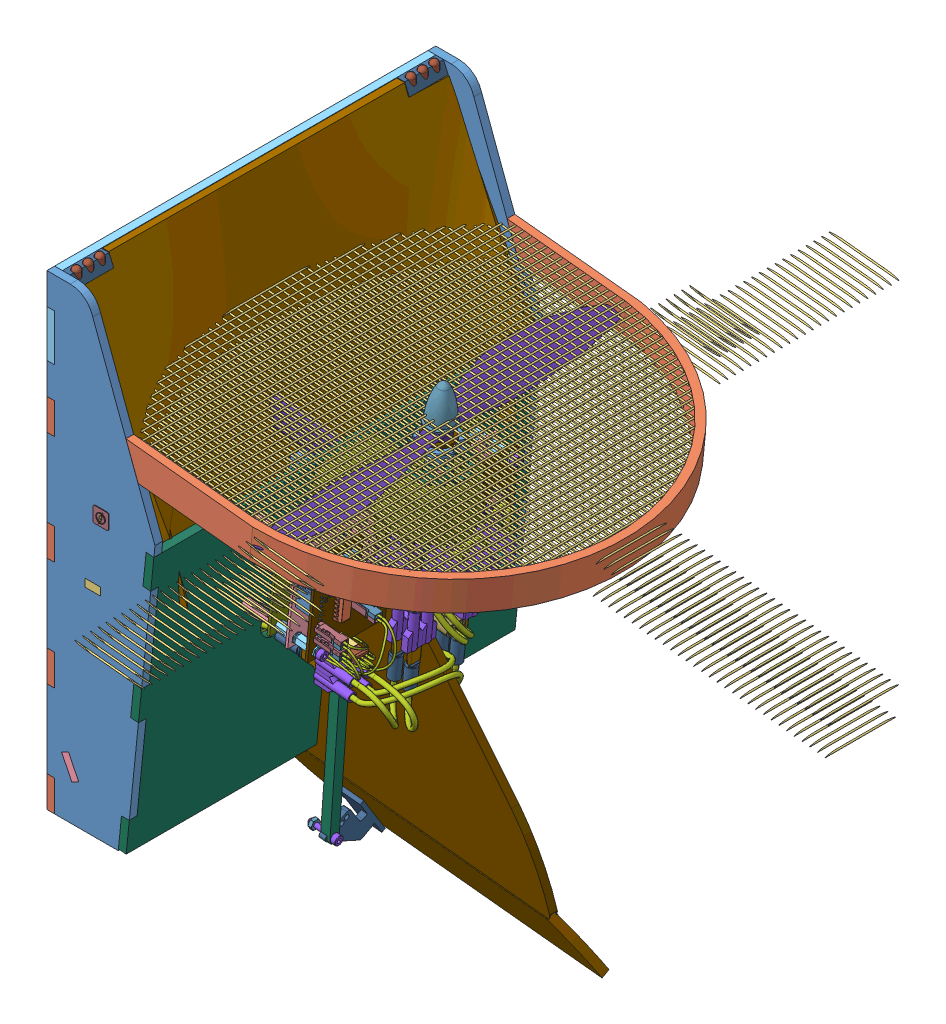
SolidWorks assembly AssTotaleSimu, configuration Défaut. Lengths in mm.
Overall size (323.53 384.35 253.57).
1760 component instances, 236 part files, 11 mates.
Components (placement in the parent):
- AssStructSimu-1: AssStructSimu [Défaut] at (-125.7658 -1.8483 624.6548) x (1 0 0) z (0 0 -1) size (323.53 326.04 251.6)
  - AssBase-1: AssBase [Défaut] at (36.5482 -71.0398 34.0612) size (266.84 303.75 251.6)
    - AssD-1: AssD [Défaut] at (39.0992 31.0201 8.5) size (69.5 300 22)
      - P1-1: P1 [Défaut] at (-95.5819 194.6656 377.5) size (69.5 300 5)
      - P5-1: P5 [Défaut] at (-100.5819 -35.3344 360.5) x (0 1 0) z (1 0 0) size (230 22 5)
    - AssG-1: AssG [Défaut] at (39.0992 31.0201 -236.5) size (69.5 300 22)
      - P1-1: P1 [Défaut] at (-95.5819 194.6656 377.5) size (69.5 300 5)
      - P5-1: P5 [Défaut] at (-95.5819 -35.3344 399.5) x (0 1 0) z (-1 0 0) size (230 22 5)
    - P7-1: P7 [Défaut] at (-1.4828 89.6857 370.5) x (0 0 -1) z (0 -1 0) size (250 54.5 5)
    - P4-1: P4 [Défaut] at (-63.2363 165.9323 386) x (0 0 -1) z (0.898794 -0.438371 0) size (250 60.5 66.27)
    - P3-1: P3 [Défaut] at (-56.4828 -74.3143 146) x (0 0 1) z (-1 0 0) size (250 70 5)
    - P4b-1: P4b [Défaut] at (-58.7423 163.7404 190) x (0 0 1) z (0.438371 0.898794 0) size (152 56 2)
    - battery-1: battery [Défaut] at (-39.0156 204.1861 197.5) x (0 0 1) z (0.898794 -0.438371 0) size (234.06 240.2 179.73)
    - socket head cap screw 4762_din-1: socket head cap screw 4762_din [EN ISO 4762 M3 x 10 - 10N] at (-27.7008 145.2627 193) x (0.438371 0.898794 0) z (0 0 -1) size (13 5.5 5.5)
    - socket head cap screw 4762_din-2: socket head cap screw 4762_din [EN ISO 4762 M3 x 10 - 10N] at (-27.7008 145.2627 339) x (0.438371 0.898794 0) z (-0.791285 0.385936 -0.474259) size (13 5.5 5.5)
    - socket head cap screw 4762_din-3: socket head cap screw 4762_din [EN ISO 4762 M3 x 10 - 10N] at (-42.0815 152.2766 339) x (0.438371 0.898794 0) z (-0.001489 0.000726 -0.999999) size (13 5.5 5.5)
    - socket head cap screw 4762_din-4: socket head cap screw 4762_din [EN ISO 4762 M3 x 10 - 10N] at (-42.0815 152.2766 193) x (0.438371 0.898794 0) z (-0.031331 0.015281 -0.999392) size (13 5.5 5.5)
    - P11-1: P11 [Défaut] at (-57.5734 -73.9703 146.7843) x (0.005072 0 0.999987) z (0.006197 0.999981 -0.000031) size (240 65 164)
    - AssPhare-1: AssPhare [Défaut] at (-52.8518 -67.6977 411) x (0 1 0) z (0 0 -1) size (43.2 8 27.06)
      - piece_led-1: piece_led [Défaut] at (-6.6166 -3.631 25) size (40.9 8 25)
      - LED 5mm-1: LED 5mm [Valor predeterminado] at (-0.1166 0.369 30) x (0 0 1) z (-1 0 0) size (5.5 6 35.8)
      - LED 5mm-2: LED 5mm [Valor predeterminado] at (-0.1166 0.369 37.5) x (0 0 1) z (-1 0 0) size (5.5 6 35.8)
      - LED 5mm-3: LED 5mm [Valor predeterminado] at (-0.1166 0.369 45) x (0 0 1) z (-1 0 0) size (5.5 6 35.8)
    - AssPhare-2: AssPhare [Défaut] at (-52.8518 -67.6977 196) x (0 1 0) z (0 0 -1) size (43.2 8 27.06)
      - piece_led-1: piece_led [Défaut] at (-6.6166 -3.631 25) size (40.9 8 25)
      - LED 5mm-1: LED 5mm [Valor predeterminado] at (-0.1166 0.369 30) x (0 0 1) z (-1 0 0) size (5.5 6 35.8)
      - LED 5mm-2: LED 5mm [Valor predeterminado] at (-0.1166 0.369 37.5) x (0 0 1) z (-1 0 0) size (5.5 6 35.8)
      - LED 5mm-3: LED 5mm [Valor predeterminado] at (-0.1166 0.369 45) x (0 0 1) z (-1 0 0) size (5.5 6 35.8)
    - AssLogo-1: AssLogo [Défaut] at (-27.8835 45.1673 148.1054) x (-1 0 0) z (0 0 -1) size (10 10 0.8)
      - logo1-1: logo1 [Défaut] at (-6.5271 -4.4734 6.5054) size (5.8 7.71 0.4)
      - logo2-1: logo2 [Défaut] at (-6.4007 -4.4815 7.1054) size (10 10 0.4)
    - AssLogo-2: AssLogo [Défaut] at (-25.082 45.1673 383.8946) size (10 10 0.8)
      - logo1-1: logo1 [Défaut] at (-6.5271 -4.4734 6.5054) size (5.8 7.71 0.4)
      - logo2-1: logo2 [Défaut] at (-6.4007 -4.4815 7.1054) size (10 10 0.4)
    - support2-1: support2 [Défaut] at (-61.5648 191.7124 276) x (-0.017452 -0.999848 0) z (0.999848 -0.017452 0) size (75 20 10) (hidden)
    - socket head cap screw 4762_din-5: socket head cap screw 4762_din [EN ISO 4762 M3 x 5 - 5N] at (-61.652 186.7132 269.3333) x (0.999848 -0.017452 0) z (-0.002158 -0.123615 0.992328) size (8 5.5 5.5)
    - socket head cap screw 4762_din-6: socket head cap screw 4762_din [EN ISO 4762 M3 x 5 - 5N] at (-61.652 186.7132 262.6667) x (0.999848 -0.017452 0) z (0 0 1) size (8 5.5 5.5)
    - socket head cap screw 4762_din-7: socket head cap screw 4762_din [EN ISO 4762 M3 x 25 - 18N] at (-55.2963 121.0922 253) x (0 0 1) z (-1 0 0) size (28 5.5 5.5)
    - hex nut style 1 gradeab_din-1: hex nut style 1 gradeab_din [Hexagon Nut ISO 4032 - M3 - W - N] at (-55.2963 121.0922 276) x (-0.923728 -0.383049 0) z (0 0 -1) size (5.5 6.35 2.4)
  - AssToitMot-1: AssToitMot [Défaut] at (-168.5238 43.6961 238.494) x (0 0 -1) z (0.9948 0.101852 0) size (250 207.5 205)
    - AssToit-1: AssToit [Défaut] at (-23.0702 -16.5789 -3.7148) size (250 207.5 205)
      - P8-1: P8 [Défaut] at (-38.4971 122.5921 203.5) size (250 175 5)
      - P12-1: P12 [Défaut] at (-60.4971 -63.4079 265.5) x (1 0 0) z (0 -1 0) size (47.03 76.64 55)
      - P13-1: P13 [Défaut] at (-35.9971 -52.8579 208.5) x (0 0 1) z (-1 0 0) size (64 15.55 5)
      - P10_2-1: P10_2 [Défaut] at (-35.9971 111.5921 171) x (0 0 1) z (-1 0 0) size (188.5 117.6 5)
    - Parallax-Servo_DUMMY-1: Parallax-Servo_DUMMY [Défaut] at (-61.6002 -51.5207 216.6662) x (1 0 0) z (0 1 0) size (20.07 42.79 55.64)
    - socket head cap screw 4762_din-1: socket head cap screw 4762_din [EN ISO 4762 M2.5 x 5 - 5N] at (-51.9272 -76.4868 259.2852) x (0 -1 0) z (-0.546944 0 0.837169) size (7.5 4.5 4.5)
    - socket head cap screw 4762_din-2: socket head cap screw 4762_din [EN ISO 4762 M2.5 x 5 - 5N] at (-61.5672 -76.4868 268.9252) x (0 -1 0) z (-0.546944 0 0.837169) size (7.5 4.5 4.5)
    - socket head cap screw 4762_din-3: socket head cap screw 4762_din [EN ISO 4762 M2.5 x 5 - 5N] at (-71.2072 -76.4868 259.2852) x (0 -1 0) z (-0.546944 0 0.837169) size (7.5 4.5 4.5)
    - socket head cap screw 4762_din-4: socket head cap screw 4762_din [EN ISO 4762 M2.5 x 5 - 5N] at (-61.5672 -76.4868 249.6452) x (0 -1 0) z (-0.546944 0 0.837169) size (7.5 4.5 4.5)
    - AssPhare-1: AssPhare [Défaut] at (8.4328 83.3966 196.1542) x (0 -1 0) z (1 0 0) size (43.2 8 27.06)
      - piece_led-1: piece_led [Défaut] at (-6.6166 -3.631 25) size (40.9 8 25)
      - LED 5mm-1: LED 5mm [Valor predeterminado] at (-0.1166 0.369 30) x (0 0 1) z (-1 0 0) size (5.5 6 35.8)
      - LED 5mm-2: LED 5mm [Valor predeterminado] at (-0.1166 0.369 37.5) x (0 0 1) z (-1 0 0) size (5.5 6 35.8)
      - LED 5mm-3: LED 5mm [Valor predeterminado] at (-0.1166 0.369 45) x (0 0 1) z (-1 0 0) size (5.5 6 35.8)
    - AssPhare-2: AssPhare [Défaut] at (-206.5672 83.3966 196.1542) x (0 -1 0) z (1 0 0) size (43.2 8 27.06)
      - piece_led-1: piece_led [Défaut] at (-6.6166 -3.631 25) size (40.9 8 25)
      - LED 5mm-1: LED 5mm [Valor predeterminado] at (-0.1166 0.369 30) x (0 0 1) z (-1 0 0) size (5.5 6 35.8)
      - LED 5mm-2: LED 5mm [Valor predeterminado] at (-0.1166 0.369 37.5) x (0 0 1) z (-1 0 0) size (5.5 6 35.8)
      - LED 5mm-3: LED 5mm [Valor predeterminado] at (-0.1166 0.369 45) x (0 0 1) z (-1 0 0) size (5.5 6 35.8)
    - socket head cap screw 4762_din-5: socket head cap screw 4762_din [EN ISO 4762 M3 x 10 - 10N] at (-67.0672 -22.9368 210.2852) x (0 0 -1) z (1 0 0) size (13 5.5 5.5)
    - socket head cap screw 4762_din-6: socket head cap screw 4762_din [EN ISO 4762 M3 x 10 - 10N] at (-56.0672 -72.9868 210.2852) x (0 0 -1) z (1 0 0) size (13 5.5 5.5)
    - socket head cap screw 4762_din-7: socket head cap screw 4762_din [EN ISO 4762 M3 x 10 - 10N] at (-67.0672 -72.9868 210.2852) x (0 0 -1) z (1 0 0) size (13 5.5 5.5)
    - socket head cap screw 4762_din-8: socket head cap screw 4762_din [EN ISO 4762 M3 x 10 - 10N] at (-56.0672 -22.9368 210.2852) x (0 0 -1) z (1 0 0) size (13 5.5 5.5)
    - hex nut style 1 gradeab_din-1: hex nut style 1 gradeab_din [Hexagon Nut ISO 4032 - M3 - W - N] at (-67.0672 -72.9868 197.3852) x (-0.923728 -0.383049 0) z (0 0 -1) size (5.5 6.35 2.4)
    - hex nut style 1 gradeab_din-2: hex nut style 1 gradeab_din [Hexagon Nut ISO 4032 - M3 - W - N] at (-56.0672 -72.9868 199.7852) size (5.5 6.35 2.4)
    - hex nut style 1 gradeab_din-3: hex nut style 1 gradeab_din [Hexagon Nut ISO 4032 - M3 - W - N] at (-67.0672 -22.9368 199.7852) size (5.5 6.35 2.4)
    - hex nut style 1 gradeab_din-4: hex nut style 1 gradeab_din [Hexagon Nut ISO 4032 - M3 - W - N] at (-56.0672 -22.9368 199.7852) size (5.5 6.35 2.4)
  - AssProtec-1: AssProtec [Défaut] at (86.6746 190.4649 284.6351) x (0 0 -1) z (0.101852 -0.9948 0) size (250 237.46 20)
    - protec3c-1: protec3c [Défaut] at (-140.4261 -87.7568 240) size (250 197 20)
    - AssGrillage-1: AssGrillage [Défaut] at (-370.4609 -132.5428 258.3161) x (0 0 -1) z (1 0 0) size (2.02 237.05 250)
      - barreau-1: barreau [Défaut] at (-1.1839 0.254 200) size (1 1 400)
      - barreau-3: barreau [Défaut] at (-1.1839 5.254 200) size (1 1 400)
      - barreau-4: barreau [Défaut] at (-1.1839 10.254 200) size (1 1 400)
      - barreau-5: barreau [Défaut] at (-1.1839 15.254 200) size (1 1 400)
      - barreau-6: barreau [Défaut] at (-1.1839 20.254 200) size (1 1 400)
      - barreau-7: barreau [Défaut] at (-1.1839 25.254 200) size (1 1 400)
      - barreau-8: barreau [Défaut] at (-1.1839 30.254 200) size (1 1 400)
      - barreau-9: barreau [Défaut] at (-1.1839 35.254 200) size (1 1 400)
      - barreau-10: barreau [Défaut] at (-1.1839 40.254 200) size (1 1 400)
      - barreau-11: barreau [Défaut] at (-1.1839 45.254 200) size (1 1 400)
      - barreau-12: barreau [Défaut] at (-1.1839 50.254 200) size (1 1 400)
      - barreau-13: barreau [Défaut] at (-1.1839 55.254 200) size (1 1 400)
      - barreau-14: barreau [Défaut] at (-1.1839 60.254 200) size (1 1 400)
      - barreau-15: barreau [Défaut] at (-1.1839 65.254 200) size (1 1 400)
      - barreau-16: barreau [Défaut] at (-1.1839 70.254 200) size (1 1 400)
      - barreau-17: barreau [Défaut] at (-1.1839 75.254 200) size (1 1 400)
      - barreau-18: barreau [Défaut] at (-1.1839 80.254 200) size (1 1 400)
      - barreau-19: barreau [Défaut] at (-1.1839 85.254 200) size (1 1 400)
      - barreau-20: barreau [Défaut] at (-1.1839 90.254 200) size (1 1 400)
      - barreau-21: barreau [Défaut] at (-1.1839 95.254 200) size (1 1 400)
      - barreau-22: barreau [Défaut] at (-1.1839 100.254 200) size (1 1 400)
      - barreau-23: barreau [Défaut] at (-1.1839 105.254 200) size (1 1 400)
      - barreau-24: barreau [Défaut] at (-1.1839 110.254 200) size (1 1 400)
      - barreau-25: barreau [Défaut] at (-1.1839 115.254 200) size (1 1 400)
      - barreau-26: barreau [Défaut] at (-1.1839 120.254 200) size (1 1 400)
      - barreau-27: barreau [Défaut] at (-1.1839 125.254 200) size (1 1 400)
      - barreau-28: barreau [Défaut] at (-1.1839 130.254 200) size (1 1 400)
      - barreau-29: barreau [Défaut] at (-1.1839 135.254 200) size (1 1 400)
      - barreau-30: barreau [Défaut] at (-1.1839 140.254 200) size (1 1 400)
      - barreau-31: barreau [Défaut] at (-1.1839 145.254 200) size (1 1 400)
      - barreau-32: barreau [Défaut] at (-1.1839 150.254 200) size (1 1 400)
      - barreau-33: barreau [Défaut] at (-1.1839 155.254 200) size (1 1 400)
      - barreau-34: barreau [Défaut] at (-1.1839 160.254 200) size (1 1 400)
      - barreau-35: barreau [Défaut] at (-1.1839 165.254 200) size (1 1 400)
      - barreau-36: barreau [Défaut] at (-1.1839 170.254 200) size (1 1 400)
      - barreau-37: barreau [Défaut] at (-1.1839 175.254 200) size (1 1 400)
      - barreau-38: barreau [Défaut] at (-1.1839 180.254 200) size (1 1 400)
      - barreau-39: barreau [Défaut] at (-1.1839 185.254 200) size (1 1 400)
      - barreau-40: barreau [Défaut] at (-1.1839 190.254 200) size (1 1 400)
      - barreau-41: barreau [Défaut] at (-1.1839 195.254 200) size (1 1 400)
      - barreau-42: barreau [Défaut] at (-0.1839 -1.5314 598.7823) x (0.998922 0 0.04641) z (0 1 0) size (1 1 400)
      - barreau-43: barreau [Défaut] at (-1.1839 200.254 200) size (1 1 400)
      - barreau-44: barreau [Défaut] at (-1.1839 205.254 200) size (1 1 400)
      - barreau-45: barreau [Défaut] at (-1.1839 210.254 200) size (1 1 400)
      - barreau-46: barreau [Défaut] at (-1.1839 215.254 200) size (1 1 400)
      - barreau-47: barreau [Défaut] at (-1.1839 220.254 200) size (1 1 400)
      - barreau-48: barreau [Défaut] at (-1.1839 225.254 200) size (1 1 400)
      - barreau-49: barreau [Défaut] at (-1.1839 230.254 200) size (1 1 400)
      - barreau-50: barreau [Défaut] at (-1.1839 235.254 200) size (1 1 400)
      - barreau-51: barreau [Défaut] at (-1.1839 240.254 200) size (1 1 400)
      - barreau-52: barreau [Défaut] at (-1.1839 245.254 200) size (1 1 400)
      - barreau-53: barreau [Défaut] at (-1.1839 250.254 200) size (1 1 400)
      - barreau-54: barreau [Défaut] at (-1.1839 255.254 200) size (1 1 400)
      - barreau-55: barreau [Défaut] at (-1.1839 260.254 200) size (1 1 400)
      - barreau-56: barreau [Défaut] at (-1.1839 265.254 200) size (1 1 400)
      - barreau-57: barreau [Défaut] at (-1.1839 270.254 200) size (1 1 400)
      - barreau-58: barreau [Défaut] at (-1.1839 275.254 200) size (1 1 400)
      - barreau-59: barreau [Défaut] at (-1.1839 280.254 200) size (1 1 400)
      - barreau-60: barreau [Défaut] at (-1.1839 285.254 200) size (1 1 400)
      - barreau-61: barreau [Défaut] at (-1.1839 290.254 200) size (1 1 400)
      - barreau-62: barreau [Défaut] at (-1.1839 295.254 200) size (1 1 400)
      - barreau-63: barreau [Défaut] at (-1.1839 300.254 200) size (1 1 400)
      - barreau-64: barreau [Défaut] at (-1.1839 305.254 200) size (1 1 400)
      - barreau-65: barreau [Défaut] at (-1.1839 310.254 200) size (1 1 400)
      - barreau-66: barreau [Défaut] at (-1.1839 315.254 200) size (1 1 400)
      - barreau-67: barreau [Défaut] at (-1.1839 320.254 200) size (1 1 400)
      - barreau-68: barreau [Défaut] at (-1.1839 325.254 200) size (1 1 400)
      - barreau-69: barreau [Défaut] at (-1.1839 330.254 200) size (1 1 400)
      - barreau-70: barreau [Défaut] at (-1.1839 335.254 200) size (1 1 400)
      - barreau-71: barreau [Défaut] at (-1.1839 340.254 200) size (1 1 400)
      - barreau-72: barreau [Défaut] at (-1.1839 345.254 200) size (1 1 400)
      - barreau-73: barreau [Défaut] at (-1.1839 350.254 200) size (1 1 400)
      - barreau-74: barreau [Défaut] at (-1.1839 355.254 200) size (1 1 400)
      - barreau-75: barreau [Défaut] at (-1.1839 360.254 200) size (1 1 400)
      - barreau-76: barreau [Défaut] at (-1.1839 365.254 200) size (1 1 400)
      - barreau-77: barreau [Défaut] at (-1.1839 370.254 200) size (1 1 400)
      - barreau-78: barreau [Défaut] at (-1.1839 375.254 200) size (1 1 400)
      - barreau-79: barreau [Défaut] at (-1.1839 380.254 200) size (1 1 400)
      - barreau-80: barreau [Défaut] at (-1.1839 385.254 200) size (1 1 400)
      - barreau-81: barreau [Défaut] at (-1.1839 390.254 200) size (1 1 400)
      - barreau-82: barreau [Défaut] at (-1.1839 395.254 200) size (1 1 400)
      - barreau-136: barreau [Défaut] at (-0.1839 -1.5314 593.7823) x (0.998922 0 0.04641) z (0 1 0) size (1 1 400)
      - barreau-137: barreau [Défaut] at (-0.1839 -1.5314 588.7823) x (0.998922 0 0.04641) z (0 1 0) size (1 1 400)
      - barreau-138: barreau [Défaut] at (-0.1839 -1.5314 583.7823) x (0.998922 0 0.04641) z (0 1 0) size (1 1 400)
      - barreau-139: barreau [Défaut] at (-0.1839 -1.5314 578.7823) x (0.998922 0 0.04641) z (0 1 0) size (1 1 400)
      - barreau-140: barreau [Défaut] at (-0.1839 -1.5314 573.7823) x (0.998922 0 0.04641) z (0 1 0) size (1 1 400)
      - barreau-141: barreau [Défaut] at (-0.1839 -1.5314 568.7823) x (0.998922 0 0.04641) z (0 1 0) size (1 1 400)
      - barreau-142: barreau [Défaut] at (-0.1839 -1.5314 563.7823) x (0.998922 0 0.04641) z (0 1 0) size (1 1 400)
      - barreau-143: barreau [Défaut] at (-0.1839 -1.5314 558.7823) x (0.998922 0 0.04641) z (0 1 0) size (1 1 400)
      - barreau-144: barreau [Défaut] at (-0.1839 -1.5314 553.7823) x (0.998922 0 0.04641) z (0 1 0) size (1 1 400)
      - barreau-145: barreau [Défaut] at (-0.1839 -1.5314 548.7823) x (0.998922 0 0.04641) z (0 1 0) size (1 1 400)
      - barreau-146: barreau [Défaut] at (-0.1839 -1.5314 543.7823) x (0.998922 0 0.04641) z (0 1 0) size (1 1 400)
      - barreau-147: barreau [Défaut] at (-0.1839 -1.5314 538.7823) x (0.998922 0 0.04641) z (0 1 0) size (1 1 400)
      - barreau-148: barreau [Défaut] at (-0.1839 -1.5314 533.7823) x (0.998922 0 0.04641) z (0 1 0) size (1 1 400)
      - barreau-149: barreau [Défaut] at (-0.1839 -1.5314 528.7823) x (0.998922 0 0.04641) z (0 1 0) size (1 1 400)
      - barreau-150: barreau [Défaut] at (-0.1839 -1.5314 523.7823) x (0.998922 0 0.04641) z (0 1 0) size (1 1 400)
      - barreau-151: barreau [Défaut] at (-0.1839 -1.5314 518.7823) x (0.998922 0 0.04641) z (0 1 0) size (1 1 400)
      - barreau-152: barreau [Défaut] at (-0.1839 -1.5314 513.7823) x (0.998922 0 0.04641) z (0 1 0) size (1 1 400)
      - barreau-153: barreau [Défaut] at (-0.1839 -1.5314 508.7823) x (0.998922 0 0.04641) z (0 1 0) size (1 1 400)
      - barreau-154: barreau [Défaut] at (-0.1839 -1.5314 503.7823) x (0.998922 0 0.04641) z (0 1 0) size (1 1 400)
      - barreau-155: barreau [Défaut] at (-0.1839 -1.5314 498.7823) x (0.998922 0 0.04641) z (0 1 0) size (1 1 400)
      - barreau-156: barreau [Défaut] at (-0.1839 -1.5314 493.7823) x (0.998922 0 0.04641) z (0 1 0) size (1 1 400)
      - barreau-157: barreau [Défaut] at (-0.1839 -1.5314 488.7823) x (0.998922 0 0.04641) z (0 1 0) size (1 1 400)
      - barreau-158: barreau [Défaut] at (-0.1839 -1.5314 483.7823) x (0.998922 0 0.04641) z (0 1 0) size (1 1 400)
      - barreau-159: barreau [Défaut] at (-0.1839 -1.5314 478.7823) x (0.998922 0 0.04641) z (0 1 0) size (1 1 400)
      - barreau-160: barreau [Défaut] at (-0.1839 -1.5314 473.7823) x (0.998922 0 0.04641) z (0 1 0) size (1 1 400)
      - barreau-161: barreau [Défaut] at (-0.1839 -1.5314 468.7823) x (0.998922 0 0.04641) z (0 1 0) size (1 1 400)
      - barreau-162: barreau [Défaut] at (-0.1839 -1.5314 463.7823) x (0.998922 0 0.04641) z (0 1 0) size (1 1 400)
      - barreau-163: barreau [Défaut] at (-0.1839 -1.5314 458.7823) x (0.998922 0 0.04641) z (0 1 0) size (1 1 400)
      - barreau-164: barreau [Défaut] at (-0.1839 -1.5314 453.7823) x (0.998922 0 0.04641) z (0 1 0) size (1 1 400)
      - barreau-165: barreau [Défaut] at (-0.1839 -1.5314 448.7823) x (0.998922 0 0.04641) z (0 1 0) size (1 1 400)
      - barreau-166: barreau [Défaut] at (-0.1839 -1.5314 443.7823) x (0.998922 0 0.04641) z (0 1 0) size (1 1 400)
      - barreau-167: barreau [Défaut] at (-0.1839 -1.5314 438.7823) x (0.998922 0 0.04641) z (0 1 0) size (1 1 400)
      - barreau-168: barreau [Défaut] at (-0.1839 -1.5314 433.7823) x (0.998922 0 0.04641) z (0 1 0) size (1 1 400)
      - barreau-169: barreau [Défaut] at (-0.1839 -1.5314 428.7823) x (0.998922 0 0.04641) z (0 1 0) size (1 1 400)
      - barreau-170: barreau [Défaut] at (-0.1839 -1.5314 423.7823) x (0.998922 0 0.04641) z (0 1 0) size (1 1 400)
      - barreau-171: barreau [Défaut] at (-0.1839 -1.5314 418.7823) x (0.998922 0 0.04641) z (0 1 0) size (1 1 400)
      - barreau-172: barreau [Défaut] at (-0.1839 -1.5314 413.7823) x (0.998922 0 0.04641) z (0 1 0) size (1 1 400)
      - barreau-173: barreau [Défaut] at (-0.1839 -1.5314 408.7823) x (0.998922 0 0.04641) z (0 1 0) size (1 1 400)
      - barreau-174: barreau [Défaut] at (-0.1839 -1.5314 403.7823) x (0.998922 0 0.04641) z (0 1 0) size (1 1 400)
      - barreau-175: barreau [Défaut] at (-0.1839 -1.5314 398.7823) x (0.998922 0 0.04641) z (0 1 0) size (1 1 400)
      - barreau-176: barreau [Défaut] at (-0.1839 -1.5314 393.7823) x (0.998922 0 0.04641) z (0 1 0) size (1 1 400)
      - barreau-177: barreau [Défaut] at (-0.1839 -1.5314 388.7823) x (0.998922 0 0.04641) z (0 1 0) size (1 1 400)
      - barreau-178: barreau [Défaut] at (-0.1839 -1.5314 383.7823) x (0.998922 0 0.04641) z (0 1 0) size (1 1 400)
      - barreau-179: barreau [Défaut] at (-0.1839 -1.5314 378.7823) x (0.998922 0 0.04641) z (0 1 0) size (1 1 400)
      - barreau-180: barreau [Défaut] at (-0.1839 -1.5314 373.7823) x (0.998922 0 0.04641) z (0 1 0) size (1 1 400)
      - barreau-181: barreau [Défaut] at (-0.1839 -1.5314 368.7823) x (0.998922 0 0.04641) z (0 1 0) size (1 1 400)
      - barreau-182: barreau [Défaut] at (-0.1839 -1.5314 363.7823) x (0.998922 0 0.04641) z (0 1 0) size (1 1 400)
      - barreau-183: barreau [Défaut] at (-0.1839 -1.5314 358.7823) x (0.998922 0 0.04641) z (0 1 0) size (1 1 400)
      - barreau-184: barreau [Défaut] at (-0.1839 -1.5314 353.7823) x (0.998922 0 0.04641) z (0 1 0) size (1 1 400)
      - barreau-185: barreau [Défaut] at (-0.1839 -1.5314 348.7823) x (0.998922 0 0.04641) z (0 1 0) size (1 1 400)
      - barreau-186: barreau [Défaut] at (-0.1839 -1.5314 343.7823) x (0.998922 0 0.04641) z (0 1 0) size (1 1 400)
      - barreau-187: barreau [Défaut] at (-0.1839 -1.5314 338.7823) x (0.998922 0 0.04641) z (0 1 0) size (1 1 400)
      - barreau-188: barreau [Défaut] at (-0.1839 -1.5314 333.7823) x (0.998922 0 0.04641) z (0 1 0) size (1 1 400)
      - barreau-189: barreau [Défaut] at (-0.1839 -1.5314 328.7823) x (0.998922 0 0.04641) z (0 1 0) size (1 1 400)
      - barreau-190: barreau [Défaut] at (-0.1839 -1.5314 323.7823) x (0.998922 0 0.04641) z (0 1 0) size (1 1 400)
      - barreau-191: barreau [Défaut] at (-0.1839 -1.5314 318.7823) x (0.998922 0 0.04641) z (0 1 0) size (1 1 400)
      - barreau-192: barreau [Défaut] at (-0.1839 -1.5314 313.7823) x (0.998922 0 0.04641) z (0 1 0) size (1 1 400)
      - barreau-193: barreau [Défaut] at (-0.1839 -1.5314 308.7823) x (0.998922 0 0.04641) z (0 1 0) size (1 1 400)
      - barreau-194: barreau [Défaut] at (-0.1839 -1.5314 303.7823) x (0.998922 0 0.04641) z (0 1 0) size (1 1 400)
      - barreau-195: barreau [Défaut] at (-0.1839 -1.5314 298.7823) x (0.998922 0 0.04641) z (0 1 0) size (1 1 400)
      - barreau-196: barreau [Défaut] at (-0.1839 -1.5314 293.7823) x (0.998922 0 0.04641) z (0 1 0) size (1 1 400)
      - barreau-197: barreau [Défaut] at (-0.1839 -1.5314 288.7823) x (0.998922 0 0.04641) z (0 1 0) size (1 1 400)
      - barreau-198: barreau [Défaut] at (-0.1839 -1.5314 283.7823) x (0.998922 0 0.04641) z (0 1 0) size (1 1 400)
      - barreau-199: barreau [Défaut] at (-0.1839 -1.5314 278.7823) x (0.998922 0 0.04641) z (0 1 0) size (1 1 400)
      - barreau-200: barreau [Défaut] at (-0.1839 -1.5314 273.7823) x (0.998922 0 0.04641) z (0 1 0) size (1 1 400)
      - barreau-201: barreau [Défaut] at (-0.1839 -1.5314 268.7823) x (0.998922 0 0.04641) z (0 1 0) size (1 1 400)
      - barreau-202: barreau [Défaut] at (-0.1839 -1.5314 263.7823) x (0.998922 0 0.04641) z (0 1 0) size (1 1 400)
      - barreau-203: barreau [Défaut] at (-0.1839 -1.5314 258.7823) x (0.998922 0 0.04641) z (0 1 0) size (1 1 400)
      - barreau-204: barreau [Défaut] at (-0.1839 -1.5314 253.7823) x (0.998922 0 0.04641) z (0 1 0) size (1 1 400)
      - barreau-205: barreau [Défaut] at (-0.1839 -1.5314 248.7823) x (0.998922 0 0.04641) z (0 1 0) size (1 1 400)
      - barreau-206: barreau [Défaut] at (-0.1839 -1.5314 243.7823) x (0.998922 0 0.04641) z (0 1 0) size (1 1 400)
      - barreau-207: barreau [Défaut] at (-0.1839 -1.5314 238.7823) x (0.998922 0 0.04641) z (0 1 0) size (1 1 400)
      - barreau-208: barreau [Défaut] at (-0.1839 -1.5314 233.7823) x (0.998922 0 0.04641) z (0 1 0) size (1 1 400)
      - barreau-209: barreau [Défaut] at (-0.1839 -1.5314 228.7823) x (0.998922 0 0.04641) z (0 1 0) size (1 1 400)
      - barreau-210: barreau [Défaut] at (-0.1839 -1.5314 223.7823) x (0.998922 0 0.04641) z (0 1 0) size (1 1 400)
      - barreau-211: barreau [Défaut] at (-0.1839 -1.5314 218.7823) x (0.998922 0 0.04641) z (0 1 0) size (1 1 400)
      - barreau-212: barreau [Défaut] at (-0.1839 -1.5314 213.7823) x (0.998922 0 0.04641) z (0 1 0) size (1 1 400)
      - barreau-213: barreau [Défaut] at (-0.1839 -1.5314 208.7823) x (0.998922 0 0.04641) z (0 1 0) size (1 1 400)
      - barreau-214: barreau [Défaut] at (-0.1839 -1.5314 203.7823) x (0.998922 0 0.04641) z (0 1 0) size (1 1 400)
    - AssGrillage-2: AssGrillage [Défaut] at (339.6086 -132.5428 241.6839) x (0 0 1) z (-1 0 0) size (2.02 237.05 250)
      - barreau-1: barreau [Défaut] at (-1.1839 0.254 200) size (1 1 400)
      - barreau-3: barreau [Défaut] at (-1.1839 5.254 200) size (1 1 400)
      - barreau-4: barreau [Défaut] at (-1.1839 10.254 200) size (1 1 400)
      - barreau-5: barreau [Défaut] at (-1.1839 15.254 200) size (1 1 400)
      - barreau-6: barreau [Défaut] at (-1.1839 20.254 200) size (1 1 400)
      - barreau-7: barreau [Défaut] at (-1.1839 25.254 200) size (1 1 400)
      - barreau-8: barreau [Défaut] at (-1.1839 30.254 200) size (1 1 400)
      - barreau-9: barreau [Défaut] at (-1.1839 35.254 200) size (1 1 400)
      - barreau-10: barreau [Défaut] at (-1.1839 40.254 200) size (1 1 400)
      - barreau-11: barreau [Défaut] at (-1.1839 45.254 200) size (1 1 400)
      - barreau-12: barreau [Défaut] at (-1.1839 50.254 200) size (1 1 400)
      - barreau-13: barreau [Défaut] at (-1.1839 55.254 200) size (1 1 400)
      - barreau-14: barreau [Défaut] at (-1.1839 60.254 200) size (1 1 400)
      - barreau-15: barreau [Défaut] at (-1.1839 65.254 200) size (1 1 400)
      - barreau-16: barreau [Défaut] at (-1.1839 70.254 200) size (1 1 400)
      - barreau-17: barreau [Défaut] at (-1.1839 75.254 200) size (1 1 400)
      - barreau-18: barreau [Défaut] at (-1.1839 80.254 200) size (1 1 400)
      - barreau-19: barreau [Défaut] at (-1.1839 85.254 200) size (1 1 400)
      - barreau-20: barreau [Défaut] at (-1.1839 90.254 200) size (1 1 400)
      - barreau-21: barreau [Défaut] at (-1.1839 95.254 200) size (1 1 400)
      - barreau-22: barreau [Défaut] at (-1.1839 100.254 200) size (1 1 400)
      - barreau-23: barreau [Défaut] at (-1.1839 105.254 200) size (1 1 400)
      - barreau-24: barreau [Défaut] at (-1.1839 110.254 200) size (1 1 400)
      - barreau-25: barreau [Défaut] at (-1.1839 115.254 200) size (1 1 400)
      - barreau-26: barreau [Défaut] at (-1.1839 120.254 200) size (1 1 400)
      - barreau-27: barreau [Défaut] at (-1.1839 125.254 200) size (1 1 400)
      - barreau-28: barreau [Défaut] at (-1.1839 130.254 200) size (1 1 400)
      - barreau-29: barreau [Défaut] at (-1.1839 135.254 200) size (1 1 400)
      - barreau-30: barreau [Défaut] at (-1.1839 140.254 200) size (1 1 400)
      - barreau-31: barreau [Défaut] at (-1.1839 145.254 200) size (1 1 400)
      - barreau-32: barreau [Défaut] at (-1.1839 150.254 200) size (1 1 400)
      - barreau-33: barreau [Défaut] at (-1.1839 155.254 200) size (1 1 400)
      - barreau-34: barreau [Défaut] at (-1.1839 160.254 200) size (1 1 400)
      - barreau-35: barreau [Défaut] at (-1.1839 165.254 200) size (1 1 400)
      - barreau-36: barreau [Défaut] at (-1.1839 170.254 200) size (1 1 400)
      - barreau-37: barreau [Défaut] at (-1.1839 175.254 200) size (1 1 400)
      - barreau-38: barreau [Défaut] at (-1.1839 180.254 200) size (1 1 400)
      - barreau-39: barreau [Défaut] at (-1.1839 185.254 200) size (1 1 400)
      - barreau-40: barreau [Défaut] at (-1.1839 190.254 200) size (1 1 400)
      - barreau-41: barreau [Défaut] at (-1.1839 195.254 200) size (1 1 400)
      - barreau-42: barreau [Défaut] at (-0.1839 -1.5314 598.7823) x (0.998922 0 0.04641) z (0 1 0) size (1 1 400)
      - barreau-43: barreau [Défaut] at (-1.1839 200.254 200) size (1 1 400)
      - barreau-44: barreau [Défaut] at (-1.1839 205.254 200) size (1 1 400)
      - barreau-45: barreau [Défaut] at (-1.1839 210.254 200) size (1 1 400)
      - barreau-46: barreau [Défaut] at (-1.1839 215.254 200) size (1 1 400)
      - barreau-47: barreau [Défaut] at (-1.1839 220.254 200) size (1 1 400)
      - barreau-48: barreau [Défaut] at (-1.1839 225.254 200) size (1 1 400)
      - barreau-49: barreau [Défaut] at (-1.1839 230.254 200) size (1 1 400)
      - barreau-50: barreau [Défaut] at (-1.1839 235.254 200) size (1 1 400)
      - barreau-51: barreau [Défaut] at (-1.1839 240.254 200) size (1 1 400)
      - barreau-52: barreau [Défaut] at (-1.1839 245.254 200) size (1 1 400)
      - barreau-53: barreau [Défaut] at (-1.1839 250.254 200) size (1 1 400)
      - barreau-54: barreau [Défaut] at (-1.1839 255.254 200) size (1 1 400)
      - barreau-55: barreau [Défaut] at (-1.1839 260.254 200) size (1 1 400)
      - barreau-56: barreau [Défaut] at (-1.1839 265.254 200) size (1 1 400)
      - barreau-57: barreau [Défaut] at (-1.1839 270.254 200) size (1 1 400)
      - barreau-58: barreau [Défaut] at (-1.1839 275.254 200) size (1 1 400)
      - barreau-59: barreau [Défaut] at (-1.1839 280.254 200) size (1 1 400)
      - barreau-60: barreau [Défaut] at (-1.1839 285.254 200) size (1 1 400)
      - barreau-61: barreau [Défaut] at (-1.1839 290.254 200) size (1 1 400)
      - barreau-62: barreau [Défaut] at (-1.1839 295.254 200) size (1 1 400)
      - barreau-63: barreau [Défaut] at (-1.1839 300.254 200) size (1 1 400)
      - barreau-64: barreau [Défaut] at (-1.1839 305.254 200) size (1 1 400)
      - barreau-65: barreau [Défaut] at (-1.1839 310.254 200) size (1 1 400)
      - barreau-66: barreau [Défaut] at (-1.1839 315.254 200) size (1 1 400)
      - barreau-67: barreau [Défaut] at (-1.1839 320.254 200) size (1 1 400)
      - barreau-68: barreau [Défaut] at (-1.1839 325.254 200) size (1 1 400)
      - barreau-69: barreau [Défaut] at (-1.1839 330.254 200) size (1 1 400)
      - barreau-70: barreau [Défaut] at (-1.1839 335.254 200) size (1 1 400)
      - barreau-71: barreau [Défaut] at (-1.1839 340.254 200) size (1 1 400)
      - barreau-72: barreau [Défaut] at (-1.1839 345.254 200) size (1 1 400)
      - barreau-73: barreau [Défaut] at (-1.1839 350.254 200) size (1 1 400)
      - barreau-74: barreau [Défaut] at (-1.1839 355.254 200) size (1 1 400)
      - barreau-75: barreau [Défaut] at (-1.1839 360.254 200) size (1 1 400)
      - barreau-76: barreau [Défaut] at (-1.1839 365.254 200) size (1 1 400)
      - barreau-77: barreau [Défaut] at (-1.1839 370.254 200) size (1 1 400)
      - barreau-78: barreau [Défaut] at (-1.1839 375.254 200) size (1 1 400)
      - barreau-79: barreau [Défaut] at (-1.1839 380.254 200) size (1 1 400)
      - barreau-80: barreau [Défaut] at (-1.1839 385.254 200) size (1 1 400)
      - barreau-81: barreau [Défaut] at (-1.1839 390.254 200) size (1 1 400)
      - barreau-82: barreau [Défaut] at (-1.1839 395.254 200) size (1 1 400)
      - barreau-136: barreau [Défaut] at (-0.1839 -1.5314 593.7823) x (0.998922 0 0.04641) z (0 1 0) size (1 1 400)
      - barreau-137: barreau [Défaut] at (-0.1839 -1.5314 588.7823) x (0.998922 0 0.04641) z (0 1 0) size (1 1 400)
      - barreau-138: barreau [Défaut] at (-0.1839 -1.5314 583.7823) x (0.998922 0 0.04641) z (0 1 0) size (1 1 400)
      - barreau-139: barreau [Défaut] at (-0.1839 -1.5314 578.7823) x (0.998922 0 0.04641) z (0 1 0) size (1 1 400)
      - barreau-140: barreau [Défaut] at (-0.1839 -1.5314 573.7823) x (0.998922 0 0.04641) z (0 1 0) size (1 1 400)
      - barreau-141: barreau [Défaut] at (-0.1839 -1.5314 568.7823) x (0.998922 0 0.04641) z (0 1 0) size (1 1 400)
      - barreau-142: barreau [Défaut] at (-0.1839 -1.5314 563.7823) x (0.998922 0 0.04641) z (0 1 0) size (1 1 400)
      - barreau-143: barreau [Défaut] at (-0.1839 -1.5314 558.7823) x (0.998922 0 0.04641) z (0 1 0) size (1 1 400)
      - barreau-144: barreau [Défaut] at (-0.1839 -1.5314 553.7823) x (0.998922 0 0.04641) z (0 1 0) size (1 1 400)
      - barreau-145: barreau [Défaut] at (-0.1839 -1.5314 548.7823) x (0.998922 0 0.04641) z (0 1 0) size (1 1 400)
      - barreau-146: barreau [Défaut] at (-0.1839 -1.5314 543.7823) x (0.998922 0 0.04641) z (0 1 0) size (1 1 400)
      - barreau-147: barreau [Défaut] at (-0.1839 -1.5314 538.7823) x (0.998922 0 0.04641) z (0 1 0) size (1 1 400)
      - barreau-148: barreau [Défaut] at (-0.1839 -1.5314 533.7823) x (0.998922 0 0.04641) z (0 1 0) size (1 1 400)
      - barreau-149: barreau [Défaut] at (-0.1839 -1.5314 528.7823) x (0.998922 0 0.04641) z (0 1 0) size (1 1 400)
      - barreau-150: barreau [Défaut] at (-0.1839 -1.5314 523.7823) x (0.998922 0 0.04641) z (0 1 0) size (1 1 400)
      - barreau-151: barreau [Défaut] at (-0.1839 -1.5314 518.7823) x (0.998922 0 0.04641) z (0 1 0) size (1 1 400)
      - barreau-152: barreau [Défaut] at (-0.1839 -1.5314 513.7823) x (0.998922 0 0.04641) z (0 1 0) size (1 1 400)
      - barreau-153: barreau [Défaut] at (-0.1839 -1.5314 508.7823) x (0.998922 0 0.04641) z (0 1 0) size (1 1 400)
      - barreau-154: barreau [Défaut] at (-0.1839 -1.5314 503.7823) x (0.998922 0 0.04641) z (0 1 0) size (1 1 400)
      - barreau-155: barreau [Défaut] at (-0.1839 -1.5314 498.7823) x (0.998922 0 0.04641) z (0 1 0) size (1 1 400)
      - barreau-156: barreau [Défaut] at (-0.1839 -1.5314 493.7823) x (0.998922 0 0.04641) z (0 1 0) size (1 1 400)
      - barreau-157: barreau [Défaut] at (-0.1839 -1.5314 488.7823) x (0.998922 0 0.04641) z (0 1 0) size (1 1 400)
      - barreau-158: barreau [Défaut] at (-0.1839 -1.5314 483.7823) x (0.998922 0 0.04641) z (0 1 0) size (1 1 400)
      - barreau-159: barreau [Défaut] at (-0.1839 -1.5314 478.7823) x (0.998922 0 0.04641) z (0 1 0) size (1 1 400)
      - barreau-160: barreau [Défaut] at (-0.1839 -1.5314 473.7823) x (0.998922 0 0.04641) z (0 1 0) size (1 1 400)
      - barreau-161: barreau [Défaut] at (-0.1839 -1.5314 468.7823) x (0.998922 0 0.04641) z (0 1 0) size (1 1 400)
      - barreau-162: barreau [Défaut] at (-0.1839 -1.5314 463.7823) x (0.998922 0 0.04641) z (0 1 0) size (1 1 400)
      - barreau-163: barreau [Défaut] at (-0.1839 -1.5314 458.7823) x (0.998922 0 0.04641) z (0 1 0) size (1 1 400)
      - barreau-164: barreau [Défaut] at (-0.1839 -1.5314 453.7823) x (0.998922 0 0.04641) z (0 1 0) size (1 1 400)
      - barreau-165: barreau [Défaut] at (-0.1839 -1.5314 448.7823) x (0.998922 0 0.04641) z (0 1 0) size (1 1 400)
      - barreau-166: barreau [Défaut] at (-0.1839 -1.5314 443.7823) x (0.998922 0 0.04641) z (0 1 0) size (1 1 400)
      - barreau-167: barreau [Défaut] at (-0.1839 -1.5314 438.7823) x (0.998922 0 0.04641) z (0 1 0) size (1 1 400)
      - barreau-168: barreau [Défaut] at (-0.1839 -1.5314 433.7823) x (0.998922 0 0.04641) z (0 1 0) size (1 1 400)
      - barreau-169: barreau [Défaut] at (-0.1839 -1.5314 428.7823) x (0.998922 0 0.04641) z (0 1 0) size (1 1 400)
      - barreau-170: barreau [Défaut] at (-0.1839 -1.5314 423.7823) x (0.998922 0 0.04641) z (0 1 0) size (1 1 400)
      - barreau-171: barreau [Défaut] at (-0.1839 -1.5314 418.7823) x (0.998922 0 0.04641) z (0 1 0) size (1 1 400)
      - barreau-172: barreau [Défaut] at (-0.1839 -1.5314 413.7823) x (0.998922 0 0.04641) z (0 1 0) size (1 1 400)
      - barreau-173: barreau [Défaut] at (-0.1839 -1.5314 408.7823) x (0.998922 0 0.04641) z (0 1 0) size (1 1 400)
      - barreau-174: barreau [Défaut] at (-0.1839 -1.5314 403.7823) x (0.998922 0 0.04641) z (0 1 0) size (1 1 400)
      - barreau-175: barreau [Défaut] at (-0.1839 -1.5314 398.7823) x (0.998922 0 0.04641) z (0 1 0) size (1 1 400)
      - barreau-176: barreau [Défaut] at (-0.1839 -1.5314 393.7823) x (0.998922 0 0.04641) z (0 1 0) size (1 1 400)
      - barreau-177: barreau [Défaut] at (-0.1839 -1.5314 388.7823) x (0.998922 0 0.04641) z (0 1 0) size (1 1 400)
      - barreau-178: barreau [Défaut] at (-0.1839 -1.5314 383.7823) x (0.998922 0 0.04641) z (0 1 0) size (1 1 400)
      - barreau-179: barreau [Défaut] at (-0.1839 -1.5314 378.7823) x (0.998922 0 0.04641) z (0 1 0) size (1 1 400)
      - barreau-180: barreau [Défaut] at (-0.1839 -1.5314 373.7823) x (0.998922 0 0.04641) z (0 1 0) size (1 1 400)
      - barreau-181: barreau [Défaut] at (-0.1839 -1.5314 368.7823) x (0.998922 0 0.04641) z (0 1 0) size (1 1 400)
      - barreau-182: barreau [Défaut] at (-0.1839 -1.5314 363.7823) x (0.998922 0 0.04641) z (0 1 0) size (1 1 400)
      - barreau-183: barreau [Défaut] at (-0.1839 -1.5314 358.7823) x (0.998922 0 0.04641) z (0 1 0) size (1 1 400)
      - barreau-184: barreau [Défaut] at (-0.1839 -1.5314 353.7823) x (0.998922 0 0.04641) z (0 1 0) size (1 1 400)
      - barreau-185: barreau [Défaut] at (-0.1839 -1.5314 348.7823) x (0.998922 0 0.04641) z (0 1 0) size (1 1 400)
      - barreau-186: barreau [Défaut] at (-0.1839 -1.5314 343.7823) x (0.998922 0 0.04641) z (0 1 0) size (1 1 400)
      - barreau-187: barreau [Défaut] at (-0.1839 -1.5314 338.7823) x (0.998922 0 0.04641) z (0 1 0) size (1 1 400)
      - barreau-188: barreau [Défaut] at (-0.1839 -1.5314 333.7823) x (0.998922 0 0.04641) z (0 1 0) size (1 1 400)
      - barreau-189: barreau [Défaut] at (-0.1839 -1.5314 328.7823) x (0.998922 0 0.04641) z (0 1 0) size (1 1 400)
      - barreau-190: barreau [Défaut] at (-0.1839 -1.5314 323.7823) x (0.998922 0 0.04641) z (0 1 0) size (1 1 400)
      - barreau-191: barreau [Défaut] at (-0.1839 -1.5314 318.7823) x (0.998922 0 0.04641) z (0 1 0) size (1 1 400)
      - barreau-192: barreau [Défaut] at (-0.1839 -1.5314 313.7823) x (0.998922 0 0.04641) z (0 1 0) size (1 1 400)
      - barreau-193: barreau [Défaut] at (-0.1839 -1.5314 308.7823) x (0.998922 0 0.04641) z (0 1 0) size (1 1 400)
      - barreau-194: barreau [Défaut] at (-0.1839 -1.5314 303.7823) x (0.998922 0 0.04641) z (0 1 0) size (1 1 400)
      - barreau-195: barreau [Défaut] at (-0.1839 -1.5314 298.7823) x (0.998922 0 0.04641) z (0 1 0) size (1 1 400)
      - barreau-196: barreau [Défaut] at (-0.1839 -1.5314 293.7823) x (0.998922 0 0.04641) z (0 1 0) size (1 1 400)
      - barreau-197: barreau [Défaut] at (-0.1839 -1.5314 288.7823) x (0.998922 0 0.04641) z (0 1 0) size (1 1 400)
      - barreau-198: barreau [Défaut] at (-0.1839 -1.5314 283.7823) x (0.998922 0 0.04641) z (0 1 0) size (1 1 400)
      - barreau-199: barreau [Défaut] at (-0.1839 -1.5314 278.7823) x (0.998922 0 0.04641) z (0 1 0) size (1 1 400)
      - barreau-200: barreau [Défaut] at (-0.1839 -1.5314 273.7823) x (0.998922 0 0.04641) z (0 1 0) size (1 1 400)
      - barreau-201: barreau [Défaut] at (-0.1839 -1.5314 268.7823) x (0.998922 0 0.04641) z (0 1 0) size (1 1 400)
      - barreau-202: barreau [Défaut] at (-0.1839 -1.5314 263.7823) x (0.998922 0 0.04641) z (0 1 0) size (1 1 400)
      - barreau-203: barreau [Défaut] at (-0.1839 -1.5314 258.7823) x (0.998922 0 0.04641) z (0 1 0) size (1 1 400)
      - barreau-204: barreau [Défaut] at (-0.1839 -1.5314 253.7823) x (0.998922 0 0.04641) z (0 1 0) size (1 1 400)
      - barreau-205: barreau [Défaut] at (-0.1839 -1.5314 248.7823) x (0.998922 0 0.04641) z (0 1 0) size (1 1 400)
      - barreau-206: barreau [Défaut] at (-0.1839 -1.5314 243.7823) x (0.998922 0 0.04641) z (0 1 0) size (1 1 400)
      - barreau-207: barreau [Défaut] at (-0.1839 -1.5314 238.7823) x (0.998922 0 0.04641) z (0 1 0) size (1 1 400)
